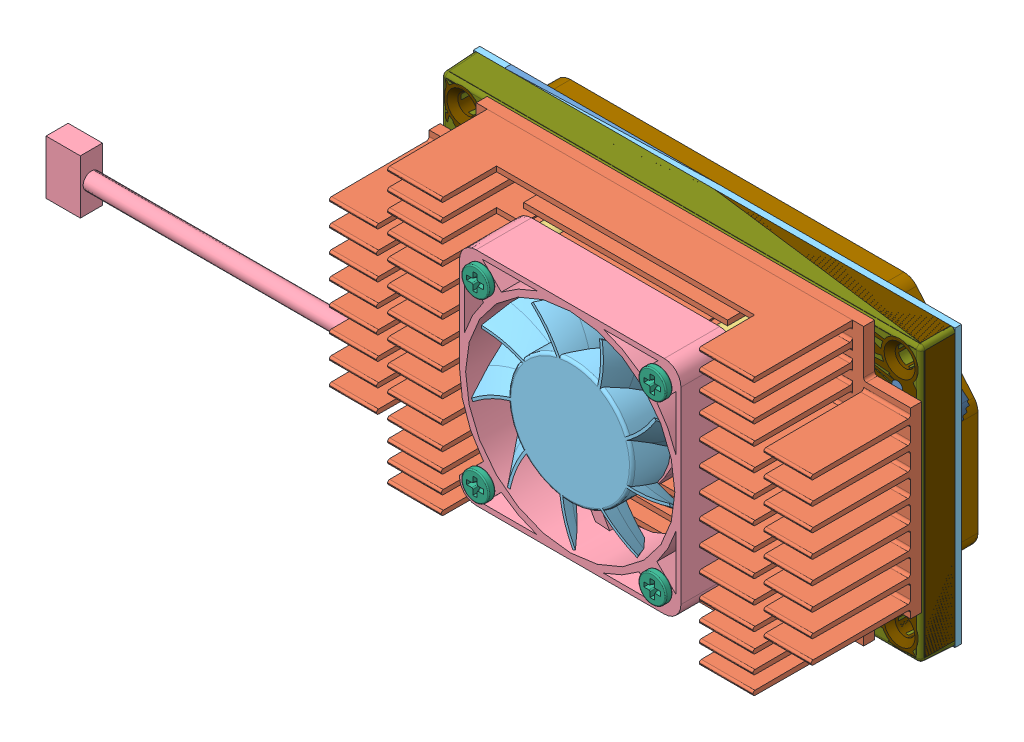
SolidWorks assembly JETSON-NEW_ASM, configuration Default. Lengths in mm. (continued)
Components (placement in the parent): (continued)
- 244-82180-1000-A03-10-12-15_ASM-1: 244-82180-1000-A03-10-12-15_ASM [Default] at origin size (87 50 8.3) (continued)
  - 039-0165-000_1-14: 039-0165-000_1 [Default] at (31.368 23.724 0) x (-1 0 0) z (0 0 -1) size (0.69 0.32 0.34)
  - 039-0165-000_1-15: 039-0165-000_1 [Default] at (30.473 23.719 0) x (-1 0 0) z (0 0 -1) size (0.69 0.32 0.34)
  - 195-2117-000_1-6: 195-2117-000_1 [Default] at (30.515 23.194 0) x (1 0 0) z (0 0 -1) size (0.69 0.32 0.31)
  - 039-0165-000_1-16: 039-0165-000_1 [Default] at (31.401 23.194 0) x (-1 0 0) z (0 0 -1) size (0.69 0.32 0.34)
  - 195-1636-000_1-21: 195-1636-000_1 [Default] at (67.75 12.2 0) x (0 -1 0) z (0 0 -1) size (0.69 0.32 0.31)
  - 039-0165-000_1-17: 039-0165-000_1 [Default] at (32.1 33 0) x (-1 0 0) z (0 0 -1) size (0.69 0.32 0.34)
  - 039-0165-000_1-18: 039-0165-000_1 [Default] at (33.713 34.804 0) x (0 1 0) z (0 0 -1) size (0.69 0.32 0.34)
  - 039-0165-000_1-19: 039-0165-000_1 [Default] at (32.583 23.814 0) x (-1 0 0) z (0 0 -1) size (0.69 0.32 0.34)
  - 039-0165-000_1-20: 039-0165-000_1 [Default] at (32.323 23.294 0) x (1 0 0) z (0 0 -1) size (0.69 0.32 0.34)
  - 195-1636-000_1-22: 195-1636-000_1 [Default] at (37.4 29.65 0) x (-1 0 0) z (0 0 -1) size (0.69 0.32 0.31)
  - 039-0165-000_1-21: 039-0165-000_1 [Default] at (11.65 14.4 0) x (1 0 0) z (0 0 -1) size (0.69 0.32 0.34)
  - 195-2006-000_1-6: 195-2006-000_1 [Default] at (11.65 13.85 0) x (1 0 0) z (0 0 -1) size (0.69 0.32 0.31)
  - 039-0165-000_1-22: 039-0165-000_1 [Default] at (32.5 41.35 0) x (0 -1 0) z (0 0 -1) size (0.69 0.32 0.34)
  - 039-0165-000_1-23: 039-0165-000_1 [Default] at (35.733 34.964 0) x (0 -1 0) z (0 0 -1) size (0.69 0.32 0.34)
  - 195-2005-000_1-8: 195-2005-000_1 [Default] at (32.265 27.36 0) x (-1 0 0) z (0 0 -1) size (0.69 0.32 0.31)
  - 195-1636-000_1-23: 195-1636-000_1 [Default] at (35.358 25.641 0) x (1 0 0) z (0 0 -1) size (0.69 0.32 0.31)
  - 039-0165-000_1-24: 039-0165-000_1 [Default] at (36.07 25.804 0) x (0 1 0) z (0 0 -1) size (0.69 0.32 0.34)
  - 039-0165-000_1-25: 039-0165-000_1 [Default] at (39.603 39.284 0) x (0 1 0) z (0 0 -1) size (0.69 0.32 0.34)
  - 039-0165-000_1-26: 039-0165-000_1 [Default] at (39.733 34.784 0) x (-1 0 0) z (0 0 -1) size (0.69 0.32 0.34)
  - 039-0165-000_1-27: 039-0165-000_1 [Default] at (40.473 23.854 0) x (0 1 0) z (0 0 -1) size (0.69 0.32 0.34)
  - 039-0165-000_1-28: 039-0165-000_1 [Default] at (37.453 39.204 0) x (-1 0 0) z (0 0 -1) size (0.69 0.32 0.34)
  - 195-1758-000_1-3: 195-1758-000_1 [Default] at (37.75 38.15 0) x (0 -1 0) z (0 0 -1) size (0.69 0.32 0.27)
  - 195-1758-000_1-4: 195-1758-000_1 [Default] at (37.8 35.75 0) x (0 -1 0) z (0 0 -1) size (0.69 0.32 0.27)
  - 039-0165-000_1-29: 039-0165-000_1 [Default] at (38.7 36 0) x (1 0 0) z (0 0 -1) size (0.69 0.32 0.34)
  - 039-0165-000_1-30: 039-0165-000_1 [Default] at (38.7 34.4 0) x (1 0 0) z (0 0 -1) size (0.69 0.32 0.34)
  - 039-0165-000_1-31: 039-0165-000_1 [Default] at (42 32.8 0) x (-1 0 0) z (0 0 -1) size (0.69 0.32 0.34)
  - 039-0165-000_1-32: 039-0165-000_1 [Default] at (39.75 33.05 0) x (0 1 0) z (0 0 -1) size (0.69 0.32 0.34)
  - 195-2005-000_1-9: 195-2005-000_1 [Default] at (40.728 29.454 0) x (0 -1 0) z (0 0 -1) size (0.69 0.32 0.31)
  - 195-1636-000_1-24: 195-1636-000_1 [Default] at (40.853 28.394 0) x (1 0 0) z (0 0 -1) size (0.69 0.32 0.31)
  - 039-0165-000_1-33: 039-0165-000_1 [Default] at (41.752 23.379 0) x (0 1 0) z (0 0 -1) size (0.69 0.32 0.34)
  - 195-2005-000_1-10: 195-2005-000_1 [Default] at (42.903 40.854 0) x (-1 0 0) z (0 0 -1) size (0.69 0.32 0.31)
  - 195-2006-000_1-7: 195-2006-000_1 [Default] at (42.753 39.054 0) x (0 -1 0) z (0 0 -1) size (0.69 0.32 0.31)
  - 195-2006-000_1-8: 195-2006-000_1 [Default] at (42.763 39.967 0) x (0 1 0) z (0 0 -1) size (0.69 0.32 0.31)
  - 039-0165-000_1-34: 039-0165-000_1 [Default] at (44.25 39.95 0) x (1 0 0) z (0 0 -1) size (0.69 0.32 0.34)
  - 039-0165-000_1-35: 039-0165-000_1 [Default] at (42.753 38.054 0) x (0 -1 0) z (0 0 -1) size (0.69 0.32 0.34)
  - 195-1636-000_1-25: 195-1636-000_1 [Default] at (42.9 35.2 0) x (0 -1 0) z (0 0 -1) size (0.69 0.32 0.31)
  - 039-0165-000_1-36: 039-0165-000_1 [Default] at (43.65 35.2 0) x (0 -1 0) z (0 0 -1) size (0.69 0.32 0.34)
  - 195-1636-000_1-26: 195-1636-000_1 [Default] at (41.4 34.05 0) x (1 0 0) z (0 0 -1) size (0.69 0.32 0.31)
  - 039-0165-000_1-37: 039-0165-000_1 [Default] at (43.7 34.15 0) x (0 -1 0) z (0 0 -1) size (0.69 0.32 0.34)
  - 039-0165-000_1-38: 039-0165-000_1 [Default] at (47.623 34.054 0) x (-1 0 0) z (0 0 -1) size (0.69 0.32 0.34)
  - 039-0165-000_1-39: 039-0165-000_1 [Default] at (48.447 33.88 0) x (0 -1 0) z (0 0 -1) size (0.69 0.32 0.34)
  - 195-2005-000_1-11: 195-2005-000_1 [Default] at (47.263 26.769 0) x (1 0 0) z (0 0 -1) size (0.69 0.32 0.31)
  - 039-0165-000_1-40: 039-0165-000_1 [Default] at (46.253 38.504 0) x (0 1 0) z (0 0 -1) size (0.69 0.32 0.34)
  - 039-0165-000_1-41: 039-0165-000_1 [Default] at (46.603 37.074 0) x (0 -1 0) z (0 0 -1) size (0.69 0.32 0.34)
  - 195-2002-000_1-1: 195-2002-000_1 [Default] at (46.55 34.9 0) x (1 0 0) z (0 0 -1) size (0.69 0.32 0.31)
  - 039-0165-000_1-42: 039-0165-000_1 [Default] at (47.15 32.9 0) x (1 0 0) z (0 0 -1) size (0.69 0.32 0.34)
  - 039-0165-000_1-43: 039-0165-000_1 [Default] at (44.25 38.9 0) x (1 0 0) z (0 0 -1) size (0.69 0.32 0.34)
  - 039-0165-000_1-44: 039-0165-000_1 [Default] at (43.853 36.604 0) x (-1 0 0) z (0 0 -1) size (0.69 0.32 0.34)
  - 039-0165-000_1-45: 039-0165-000_1 [Default] at (45.353 34.444 0) x (-1 0 0) z (0 0 -1) size (0.69 0.32 0.34)
  - 039-0165-000_1-46: 039-0165-000_1 [Default] at (45.5 32.55 0) x (0 -1 0) z (0 0 -1) size (0.69 0.32 0.34)
  - 039-0165-000_1-47: 039-0165-000_1 [Default] at (43.65 33.05 0) x (0 1 0) z (0 0 -1) size (0.69 0.32 0.34)
  - 195-1636-000_1-27: 195-1636-000_1 [Default] at (48.94 10.93 0) x (0 -1 0) z (0 0 -1) size (0.69 0.32 0.31)
  - 039-0165-000_1-48: 039-0165-000_1 [Default] at (50.928 40.754 0) x (1 0 0) z (0 0 -1) size (0.69 0.32 0.34)
  - 039-0165-000_1-49: 039-0165-000_1 [Default] at (49.163 33.855 0) x (0 -1 0) z (0 0 -1) size (0.69 0.32 0.34)
  - 039-0165-000_1-50: 039-0165-000_1 [Default] at (51.243 29.284 0) x (1 0 0) z (0 0 -1) size (0.69 0.32 0.34)
  - 039-0165-000_1-51: 039-0165-000_1 [Default] at (50.503 39.654 0) x (-1 0 0) z (0 0 -1) size (0.69 0.32 0.34)
  - 039-0165-000_1-52: 039-0165-000_1 [Default] at (50.503 38.954 0) x (-1 0 0) z (0 0 -1) size (0.69 0.32 0.34)
  - 039-0165-000_1-53: 039-0165-000_1 [Default] at (49.853 36.179 0) x (0 1 0) z (0 0 -1) size (0.69 0.32 0.34)
  - 039-0165-000_1-54: 039-0165-000_1 [Default] at (50.314 37.05 0) x (-1 0 0) z (0 0 -1) size (0.69 0.32 0.34)
  - 195-2002-000_1-2: 195-2002-000_1 [Default] at (47.45 34.9 0) x (-1 0 0) z (0 0 -1) size (0.69 0.32 0.31)
  - 039-0165-000_1-55: 039-0165-000_1 [Default] at (48.879 32.877 0) x (-1 0 0) z (0 0 -1) size (0.69 0.32 0.34)
  - 195-1636-000_1-28: 195-1636-000_1 [Default] at (48.34 10.93 0) x (0 -1 0) z (0 0 -1) size (0.69 0.32 0.31)
  - 035-0122-000_1-1: 035-0122-000_1 [Default] at (4.828 35.604 1.164) x (0 1 0) z (0 0 1) size (0.69 0.32 0.34)
  - 195-1636-000_1-29: 195-1636-000_1 [Default] at (4.753 32.979 1.164) x (-1 0 0) z (0 0 1) size (0.69 0.32 0.31)
  - 195-1636-000_1-30: 195-1636-000_1 [Default] at (4.512 32.738 1.164) x (0 1 0) z (0 0 1) size (0.69 0.32 0.31)
  - 035-0122-000_1-2: 035-0122-000_1 [Default] at (4.078 33.854 1.164) x (-1 0 0) z (0 0 1) size (0.69 0.32 0.34)
  - 195-1636-000_1-31: 195-1636-000_1 [Default] at (5.061 30.945 1.164) x (-1 0 0) z (0 0 1) size (0.69 0.32 0.31)
  - 130-0330-000_1-1: 130-0330-000_1 [Default] at (4.408 29.445 1.164) x (0 -1 0) z (0 0 1) size (0.69 0.32 0.34)
  - 035-0243-000_2-4: 035-0243-000_2 [Default] at (5.191 29.686 1.164) x (-1 0 0) z (0 0 1) size (0.69 0.32 0.34)
  - 195-2005-000_1-12: 195-2005-000_1 [Default] at (5.423 27.972 1.164) x (0 -1 0) z (0 0 1) size (0.69 0.32 0.31)
  - 195-2005-000_1-13: 195-2005-000_1 [Default] at (4.705 27.972 1.164) x (0 -1 0) z (0 0 1) size (0.69 0.32 0.31)
  - 039-0165-000_1-56: 039-0165-000_1 [Default] at (18.95 30.45 0) x (-1 0 0) z (0 0 -1) size (0.69 0.32 0.34)
  - 130-0330-000_1-2: 130-0330-000_1 [Default] at (3.596 35.184 1.164) x (-1 0 0) z (0 0 1) size (0.69 0.32 0.34)
  - 195-1636-000_1-32: 195-1636-000_1 [Default] at (4.533 25.324 1.164) x (0 1 0) z (0 0 1) size (0.69 0.32 0.31)
  - 035-0243-000_2-5: 035-0243-000_2 [Default] at (8.235 29.188 1.164) x (-1 0 0) z (0 0 1) size (0.69 0.32 0.34)
  - 195-2005-000_1-14: 195-2005-000_1 [Default] at (8.218 25.314 1.164) x (0 -1 0) z (0 0 1) size (0.69 0.32 0.31)
  - 195-1636-000_1-33: 195-1636-000_1 [Default] at (7.7 25.314 1.164) x (0 1 0) z (0 0 1) size (0.69 0.32 0.31)
  - 195-1636-000_1-34: 195-1636-000_1 [Default] at (8.736 25.314 1.164) x (0 1 0) z (0 0 1) size (0.69 0.32 0.31)
  - 195-1636-000_1-35: 195-1636-000_1 [Default] at (5.814 36.455 1.164) x (-1 0 0) z (0 0 1) size (0.69 0.32 0.31)
  - 035-0243-000_2-6: 035-0243-000_2 [Default] at (6.599 34.734 1.164) x (-1 0 0) z (0 0 1) size (0.69 0.32 0.34)
  - 035-0243-000_2-7: 035-0243-000_2 [Default] at (5.823 35.854 1.164) x (-1 0 0) z (0 0 1) size (0.69 0.32 0.34)
  - 195-1636-000_1-36: 195-1636-000_1 [Default] at (6.723 35.854 1.164) x (-1 0 0) z (0 0 1) size (0.69 0.32 0.31)
  - 035-0243-000_2-8: 035-0243-000_2 [Default] at (6.599 33.749 1.164) x (-1 0 0) z (0 0 1) size (0.69 0.32 0.34)
  - 035-0243-000_2-9: 035-0243-000_2 [Default] at (6.51 31.341 1.164) size (0.69 0.32 0.34)
  - 035-0243-000_2-10: 035-0243-000_2 [Default] at (6.787 32.049 1.164) x (0 -1 0) z (0 0 1) size (0.69 0.32 0.34)
  - 195-1636-000_1-37: 195-1636-000_1 [Default] at (6.269 32.049 1.164) x (0 -1 0) z (0 0 1) size (0.69 0.32 0.31)
  - 035-0122-000_1-3: 035-0122-000_1 [Default] at (5.803 30.204 1.164) x (-1 0 0) z (0 0 1) size (0.69 0.32 0.34)
  - 035-0122-000_1-4: 035-0122-000_1 [Default] at (5.703 29.004 1.164) x (-1 0 0) z (0 0 1) size (0.69 0.32 0.34)
  - 195-2005-000_1-15: 195-2005-000_1 [Default] at (6.108 27.972 1.164) x (0 -1 0) z (0 0 1) size (0.69 0.32 0.31)
  - 039-0165-000_1-57: 039-0165-000_1 [Default] at (9.35 17.8 0) x (0 -1 0) z (0 0 -1) size (0.69 0.32 0.34)
  - 195-1636-000_1-38: 195-1636-000_1 [Default] at (6.146 25.314 1.164) x (0 1 0) z (0 0 1) size (0.69 0.32 0.31)
  - 195-1636-000_1-39: 195-1636-000_1 [Default] at (6.664 25.314 1.164) x (0 1 0) z (0 0 1) size (0.69 0.32 0.31)
  - 195-1636-000_1-40: 195-1636-000_1 [Default] at (7.182 25.314 1.164) x (0 1 0) z (0 0 1) size (0.69 0.32 0.31)
  - 195-1636-000_1-41: 195-1636-000_1 [Default] at (5.628 25.314 1.164) x (0 1 0) z (0 0 1) size (0.69 0.32 0.31)
  - 195-2006-000_1-9: 195-2006-000_1 [Default] at (17.687 31.24 0) x (0 -1 0) z (0 0 -1) size (0.69 0.32 0.31)
  - 195-1636-000_1-42: 195-1636-000_1 [Default] at (5.103 37.229 1.164) x (0 -1 0) z (0 0 1) size (0.69 0.32 0.31)
  - 195-1636-000_1-43: 195-1636-000_1 [Default] at (5.103 36.747 1.164) x (0 1 0) z (0 0 1) size (0.69 0.32 0.31)
  - 035-0243-000_2-11: 035-0243-000_2 [Default] at (4.078 34.434 1.164) x (-1 0 0) z (0 0 1) size (0.69 0.32 0.34)
  - 130-0334-000_1-1: 130-0334-000_1 [Default] at (9.408 35.498 1.164) x (0 -1 0) z (0 0 1) size (0.69 0.32 0.34)
  - 035-0105-000_1-1: 035-0105-000_1 [Default] at (10.11 35.738 1.164) size (0.69 0.32 0.34)
  - 130-0280-000_1-1: 130-0280-000_1 [Default] at (9.959 34.495 1.164) x (0 -1 0) z (0 0 1) size (0.69 0.32 0.36)
  - 035-0105-000_1-2: 035-0105-000_1 [Default] at (8.706 35.739 1.164) size (0.69 0.32 0.34)
  - 130-0330-000_1-3: 130-0330-000_1 [Default] at (9.78 32.603 1.164) x (0 -1 0) z (0 0 1) size (0.69 0.32 0.34)
  - 035-0243-000_2-12: 035-0243-000_2 [Default] at (10.088 33.749 1.164) x (-1 0 0) z (0 0 1) size (0.69 0.32 0.34)
  - 130-0330-000_1-4: 130-0330-000_1 [Default] at (9.381 33.989 1.164) x (0 1 0) z (0 0 1) size (0.69 0.32 0.34)
  - 035-0105-000_1-3: 035-0105-000_1 [Default] at (9.009 32.844 1.164) size (0.69 0.32 0.34)
  - 035-0105-000_1-4: 035-0105-000_1 [Default] at (10.39 32.142 1.164) x (0 1 0) z (0 0 1) size (0.69 0.32 0.34)
  - 130-0334-000_1-2: 130-0334-000_1 [Default] at (9.861 31.66 1.164) x (0 -1 0) z (0 0 1) size (0.69 0.32 0.34)
  - 035-0105-000_1-5: 035-0105-000_1 [Default] at (9.343 31.66 1.164) x (0 1 0) z (0 0 1) size (0.69 0.32 0.34)
  - 130-0330-000_1-5: 130-0330-000_1 [Default] at (9.602 29.429 1.164) x (0 1 0) z (0 0 1) size (0.69 0.32 0.34)
  - 195-2005-000_1-16: 195-2005-000_1 [Default] at (10.223 27.779 1.164) size (0.69 0.32 0.31)
  - 195-1636-000_1-44: 195-1636-000_1 [Default] at (9.254 25.314 1.164) x (0 1 0) z (0 0 1) size (0.69 0.32 0.31)
  - 035-0122-000_1-5: 035-0122-000_1 [Default] at (7.483 37.064 1.164) x (0 -1 0) z (0 0 1) size (0.69 0.32 0.34)
  - 035-0243-000_2-13: 035-0243-000_2 [Default] at (7.483 35.613 1.164) x (0 -1 0) z (0 0 1) size (0.69 0.32 0.34)
  - 130-0298-000_1-2: 130-0298-000_1 [Default] at (8.358 34.495 1.164) x (0 -1 0) z (0 0 1) size (0.69 0.32 0.36)
  - 035-0122-000_1-6: 035-0122-000_1 [Default] at (8.004 35.549 1.164) x (0 -1 0) z (0 0 1) size (0.69 0.32 0.34)
  - 035-0122-000_1-7: 035-0122-000_1 [Default] at (8.043 32.844 1.164) size (0.69 0.32 0.34)
  - 035-0122-000_1-8: 035-0122-000_1 [Default] at (7.235 30.984 1.164) x (0 -1 0) z (0 0 1) size (0.69 0.32 0.34)
  - 035-0122-000_1-9: 035-0122-000_1 [Default] at (7.305 32.049 1.164) x (0 1 0) z (0 0 1) size (0.69 0.32 0.34)
  - 035-0243-000_2-14: 035-0243-000_2 [Default] at (8.235 30.222 1.164) x (-1 0 0) z (0 0 1) size (0.69 0.32 0.34)
  - 035-0122-000_1-10: 035-0122-000_1 [Default] at (10.495 37.647 1.164) size (0.69 0.32 0.34)
  - 035-0122-000_1-11: 035-0122-000_1 [Default] at (10.495 37.129 1.164) size (0.69 0.32 0.34)
  - 035-0105-000_1-6: 035-0105-000_1 [Default] at (10.562 32.844 1.164) size (0.69 0.32 0.34)
  - 039-0165-000_1-58: 039-0165-000_1 [Default] at (11.078 33.679 1.164) x (0 1 0) z (0 0 1) size (0.69 0.32 0.34)
  - 035-0243-000_2-15: 035-0243-000_2 [Default] at (10.523 29.188 1.164) x (-1 0 0) z (0 0 1) size (0.69 0.32 0.34)
  - 195-2337-000_1-1: 195-2337-000_1 [Default] at (14.912 30.106 1.164) x (0 1 0) z (0 0 1) size (0.69 0.32 0.31)
  - 035-0135-000_1-1: 035-0135-000_1 [Default] at (14.93 29.21 1.164) x (0 -1 0) z (0 0 1) size (0.69 0.32 0.34)
  - 195-2005-000_1-17: 195-2005-000_1 [Default] at (13.85 41.55 0) x (0 -1 0) z (0 0 -1) size (0.69 0.32 0.31)
  - 039-0165-000_1-59: 039-0165-000_1 [Default] at (13.85 40.55 0) x (0 -1 0) z (0 0 -1) size (0.69 0.32 0.34)
  - 035-0105-000_1-7: 035-0105-000_1 [Default] at (13.573 36.209 1.164) x (0 -1 0) z (0 0 1) size (0.69 0.32 0.34)
  - 035-0105-000_1-8: 035-0105-000_1 [Default] at (12.753 37.409 1.164) size (0.69 0.32 0.34)
  - 195-1636-000_1-45: 195-1636-000_1 [Default] at (13.621 34.372 0) x (0 1 0) z (0 0 -1) size (0.69 0.32 0.31)
  - 035-0135-000_1-2: 035-0135-000_1 [Default] at (13.038 28.694 1.164) x (-1 0 0) z (0 0 1) size (0.69 0.32 0.34)
  - 035-0234-000_2-1: 035-0234-000_2 [Default] at (14.085 37.68 1.164) x (-1 0 0) z (0 0 1) size (0.69 0.32 0.34)
  - 035-0122-000_1-12: 035-0122-000_1 [Default] at (14.106 36.209 1.164) x (0 1 0) z (0 0 1) size (0.69 0.32 0.34)
  - 130-0330-000_1-6: 130-0330-000_1 [Default] at (13.817 36.938 1.164) size (0.69 0.32 0.34)
  - 035-0122-000_1-13: 035-0122-000_1 [Default] at (15.525 36.204 1.164) x (0 1 0) z (0 0 1) size (0.69 0.32 0.34)
  - 039-0165-000_1-60: 039-0165-000_1 [Default] at (15.007 36.204 1.164) x (0 1 0) z (0 0 1) size (0.69 0.32 0.34)
  - 195-1636-000_1-46: 195-1636-000_1 [Default] at (17.087 17.723 0) x (1 0 0) z (0 0 -1) size (0.69 0.32 0.31)
  - 195-1636-000_1-47: 195-1636-000_1 [Default] at (17.1 16.02 0) x (1 0 0) z (0 0 -1) size (0.69 0.32 0.31)
  - 195-1636-000_1-48: 195-1636-000_1 [Default] at (17.05 16.57 0) x (1 0 0) z (0 0 -1) size (0.69 0.32 0.31)
  - 039-0165-000_1-61: 039-0165-000_1 [Default] at (15.397 32.956 0) x (0 -1 0) z (0 0 -1) size (0.69 0.32 0.34)
  - 039-0165-000_1-62: 039-0165-000_1 [Default] at (16.621 39.105 0) x (0 1 0) z (0 0 -1) size (0.69 0.32 0.34)
  - 195-2005-000_1-18: 195-2005-000_1 [Default] at (16.063 36.204 1.164) x (0 1 0) z (0 0 1) size (0.69 0.32 0.31)
  - 195-1636-000_1-49: 195-1636-000_1 [Default] at (17.087 18.25 0) x (1 0 0) z (0 0 -1) size (0.69 0.32 0.31)
  - 039-0199-000_1-1: 039-0199-000_1 [Default] at (16.451 29.906 1.164) x (0 -1 0) z (0 0 1) size (0.69 0.32 0.36)
  - 195-2117-000_1-7: 195-2117-000_1 [Default] at (19.3 11.7 0) x (0 1 0) z (0 0 -1) size (0.69 0.32 0.31)
  - 195-2117-000_1-8: 195-2117-000_1 [Default] at (18.55 17.19 0) x (1 0 0) z (0 0 -1) size (0.69 0.32 0.31)
  - 195-2005-000_1-19: 195-2005-000_1 [Default] at (18.588 36.204 1.164) x (0 1 0) z (0 0 1) size (0.69 0.32 0.31)
  - 195-1636-000_1-50: 195-1636-000_1 [Default] at (17.853 36.204 1.164) x (0 -1 0) z (0 0 1) size (0.69 0.32 0.31)
  - 195-1636-000_1-51: 195-1636-000_1 [Default] at (18.597 34.602 0) x (0 1 0) z (0 0 -1) size (0.69 0.32 0.31)
  - 195-1636-000_1-52: 195-1636-000_1 [Default] at (18.079 34.602 0) x (0 1 0) z (0 0 -1) size (0.69 0.32 0.31)
  - 195-1636-000_1-53: 195-1636-000_1 [Default] at (17.409 34.602 0) x (0 1 0) z (0 0 -1) size (0.69 0.32 0.31)
  - 195-2172-000_1-1: 195-2172-000_1 [Default] at (27.7 14.4 1.164) x (-1 0 0) z (0 0 1) size (0.69 0.32 0.31)
  - 195-2172-000_1-2: 195-2172-000_1 [Default] at (27.723 12.914 1.164) x (-1 0 0) z (0 0 1) size (0.69 0.32 0.31)
  - 195-2487-000_1-1: 195-2487-000_1 [Default] at (26.123 16.104 0) x (0 1 0) z (0 0 -1) size (0.69 0.32 0.31)
  - 195-2006-000_1-10: 195-2006-000_1 [Default] at (24.965 11.846 0) x (0 -1 0) z (0 0 -1) size (0.69 0.32 0.31)
  - 039-0165-000_1-63: 039-0165-000_1 [Default] at (12.35 19.25 0) x (-1 0 0) z (0 0 -1) size (0.69 0.32 0.34)
  - 039-0165-000_1-64: 039-0165-000_1 [Default] at (7.6 21.05 0) x (1 0 0) z (0 0 -1) size (0.69 0.32 0.34)
  - 035-0243-000_2-16: 035-0243-000_2 [Default] at (27.7 21.95 1.164) size (0.69 0.32 0.34)
  - 195-2506-000_1-3: 195-2506-000_1 [Default] at (27.7 16.9 1.164) x (-1 0 0) z (0 0 1) size (0.69 0.32 0.31)
  - 039-0165-000_1-65: 039-0165-000_1 [Default] at (31.213 15.274 0) x (1 0 0) z (0 0 -1) size (0.69 0.32 0.34)
  - 039-0165-000_1-66: 039-0165-000_1 [Default] at (31.903 14.494 0) x (0 1 0) z (0 0 -1) size (0.69 0.32 0.34)
  - 039-0165-000_1-67: 039-0165-000_1 [Default] at (31.183 14.754 0) x (-1 0 0) z (0 0 -1) size (0.69 0.32 0.34)
  - 039-0165-000_1-68: 039-0165-000_1 [Default] at (31.133 14.234 0) x (-1 0 0) z (0 0 -1) size (0.69 0.32 0.34)
  - 039-0165-000_1-69: 039-0165-000_1 [Default] at (31.713 13.704 0) x (-1 0 0) z (0 0 -1) size (0.69 0.32 0.34)
  - 035-0243-000_2-17: 035-0243-000_2 [Default] at (32.85 8.65 1.164) size (0.69 0.32 0.34)
  - 039-0165-000_1-70: 039-0165-000_1 [Default] at (30.533 21.774 0) x (1 0 0) z (0 0 -1) size (0.69 0.32 0.34)
  - 195-2004-000_1-1: 195-2004-000_1 [Default] at (30.109 20.345 0) x (1 0 0) z (0 0 -1) size (0.69 0.32 0.31)
  - 195-1636-000_1-54: 195-1636-000_1 [Default] at (30.003 19.574 0) x (0 1 0) z (0 0 -1) size (0.69 0.32 0.31)
  - 039-0165-000_1-71: 039-0165-000_1 [Default] at (34.778 14.474 0) x (0 1 0) z (0 0 -1) size (0.69 0.32 0.34)
  - 039-0165-000_1-72: 039-0165-000_1 [Default] at (35.296 14.474 0) x (0 1 0) z (0 0 -1) size (0.69 0.32 0.34)
  - 039-0165-000_1-73: 039-0165-000_1 [Default] at (32.323 22.184 0) x (1 0 0) z (0 0 -1) size (0.69 0.32 0.34)
  - 039-0165-000_1-74: 039-0165-000_1 [Default] at (32.323 21.124 0) x (1 0 0) z (0 0 -1) size (0.69 0.32 0.34)
  - 039-0165-000_1-75: 039-0165-000_1 [Default] at (32.323 21.644 0) x (1 0 0) z (0 0 -1) size (0.69 0.32 0.34)
  - 039-0165-000_1-76: 039-0165-000_1 [Default] at (32.323 20.034 0) x (1 0 0) z (0 0 -1) size (0.69 0.32 0.34)
  - 039-0165-000_1-77: 039-0165-000_1 [Default] at (32.323 20.564 0) x (1 0 0) z (0 0 -1) size (0.69 0.32 0.34)
  - 039-0165-000_1-78: 039-0165-000_1 [Default] at (32.323 19.514 0) x (1 0 0) z (0 0 -1) size (0.69 0.32 0.34)
  - 039-0165-000_1-79: 039-0165-000_1 [Default] at (32.323 17.394 0) x (1 0 0) z (0 0 -1) size (0.69 0.32 0.34)
  - 039-0165-000_1-80: 039-0165-000_1 [Default] at (32.323 16.794 0) x (1 0 0) z (0 0 -1) size (0.69 0.32 0.34)
  - 039-0165-000_1-81: 039-0165-000_1 [Default] at (32.323 16.274 0) x (1 0 0) z (0 0 -1) size (0.69 0.32 0.34)
  - 039-0165-000_1-82: 039-0165-000_1 [Default] at (32.323 15.744 0) x (1 0 0) z (0 0 -1) size (0.69 0.32 0.34)
  - 039-0165-000_1-83: 039-0165-000_1 [Default] at (32.323 15.214 0) x (1 0 0) z (0 0 -1) size (0.69 0.32 0.34)
  - 039-0165-000_1-84: 039-0165-000_1 [Default] at (32.954 14.494 0) x (0 1 0) z (0 0 -1) size (0.69 0.32 0.34)
  - 039-0165-000_1-85: 039-0165-000_1 [Default] at (32.436 14.494 0) x (0 1 0) z (0 0 -1) size (0.69 0.32 0.34)
  - 195-2172-000_1-3: 195-2172-000_1 [Default] at (34.65 10.1 1.164) x (0 -1 0) z (0 0 1) size (0.69 0.32 0.31)
  - 035-0243-000_2-18: 035-0243-000_2 [Default] at (33.323 10.09 1.164) x (0 1 0) z (0 0 1) size (0.69 0.32 0.34)
  - 039-0165-000_1-86: 039-0165-000_1 [Default] at (31.433 21.764 0) x (-1 0 0) z (0 0 -1) size (0.69 0.32 0.34)
  - 039-0165-000_1-87: 039-0165-000_1 [Default] at (32.323 22.724 0) x (1 0 0) z (0 0 -1) size (0.69 0.32 0.34)
  - 039-0165-000_1-88: 039-0165-000_1 [Default] at (31.363 20.344 0) x (-1 0 0) z (0 0 -1) size (0.69 0.32 0.34)
  - 039-0165-000_1-89: 039-0165-000_1 [Default] at (38.068 14.474 0) x (0 1 0) z (0 0 -1) size (0.69 0.32 0.34)
  - 039-0165-000_1-90: 039-0165-000_1 [Default] at (37.55 14.474 0) x (0 1 0) z (0 0 -1) size (0.69 0.32 0.34)
  - 039-0165-000_1-91: 039-0165-000_1 [Default] at (38.586 14.474 0) x (0 1 0) z (0 0 -1) size (0.69 0.32 0.34)
  - 039-0165-000_1-92: 039-0165-000_1 [Default] at (39.104 14.474 0) x (0 1 0) z (0 0 -1) size (0.69 0.32 0.34)
  - 195-2631-000_1-1: 195-2631-000_1 [Default] at (38.639 10.011 1.164) x (0 -1 0) z (0 0 1) size (0.69 0.32 0.31)
  - 195-1636-000_1-55: 195-1636-000_1 [Default] at (38.36 9.734 1.164) x (-1 0 0) z (0 0 1) size (0.69 0.32 0.31)
  - 195-1636-000_1-56: 195-1636-000_1 [Default] at (38.36 10.292 1.164) x (-1 0 0) z (0 0 1) size (0.69 0.32 0.31)
  - 039-0165-000_1-93: 039-0165-000_1 [Default] at (35.814 14.474 0) x (0 1 0) z (0 0 -1) size (0.69 0.32 0.34)
  - 039-0165-000_1-94: 039-0165-000_1 [Default] at (34.172 14.474 0) x (0 1 0) z (0 0 -1) size (0.69 0.32 0.34)
  - 039-0165-000_1-95: 039-0165-000_1 [Default] at (40.833 17.074 0) x (-1 0 0) z (0 0 -1) size (0.69 0.32 0.34)
  - 039-0165-000_1-96: 039-0165-000_1 [Default] at (40.833 16.034 0) x (-1 0 0) z (0 0 -1) size (0.69 0.32 0.34)
  - 039-0165-000_1-97: 039-0165-000_1 [Default] at (40.833 15.514 0) x (-1 0 0) z (0 0 -1) size (0.69 0.32 0.34)
  - 039-0165-000_1-98: 039-0165-000_1 [Default] at (40.843 14.994 0) x (-1 0 0) z (0 0 -1) size (0.69 0.32 0.34)
  - 039-0165-000_1-99: 039-0165-000_1 [Default] at (40.843 14.474 0) x (-1 0 0) z (0 0 -1) size (0.69 0.32 0.34)
  - 039-0165-000_1-100: 039-0165-000_1 [Default] at (42.073 13.724 0) x (0 1 0) z (0 0 -1) size (0.69 0.32 0.34)
  - 039-0165-000_1-101: 039-0165-000_1 [Default] at (41.553 13.724 0) x (0 -1 0) z (0 0 -1) size (0.69 0.32 0.34)
  - 039-0165-000_1-102: 039-0165-000_1 [Default] at (41.033 13.724 0) x (0 -1 0) z (0 0 -1) size (0.69 0.32 0.34)
  - 195-2363-000_1-1: 195-2363-000_1 [Default] at (40.25 10.1 1.164) x (0 -1 0) z (0 0 1) size (0.69 0.32 0.31)
  - 195-2631-000_1-2: 195-2631-000_1 [Default] at (41.863 10.104 1.164) x (0 1 0) z (0 0 1) size (0.69 0.32 0.31)
  - 195-1636-000_1-57: 195-1636-000_1 [Default] at (10.8 12.1 0) x (0 -1 0) z (0 0 -1) size (0.69 0.32 0.31)
  - 039-0165-000_1-103: 039-0165-000_1 [Default] at (40.14 14.474 0) x (0 1 0) z (0 0 -1) size (0.69 0.32 0.34)
  - 039-0165-000_1-104: 039-0165-000_1 [Default] at (39.622 14.474 0) x (0 1 0) z (0 0 -1) size (0.69 0.32 0.34)
  - 195-2631-000_1-3: 195-2631-000_1 [Default] at (39.729 10.094 1.164) x (0 -1 0) z (0 0 1) size (0.69 0.32 0.31)
  - 039-0165-000_1-105: 039-0165-000_1 [Default] at (64.72 13.486 0) x (0 -1 0) z (0 0 -1) size (0.69 0.32 0.34)
  - 195-1636-000_1-58: 195-1636-000_1 [Default] at (43.938 22.284 0) x (0 1 0) z (0 0 -1) size (0.69 0.32 0.31)
  - 195-2363-000_1-2: 195-2363-000_1 [Default] at (42.35 11.2 0) x (0 -1 0) z (0 0 -1) size (0.69 0.32 0.31)
  - 195-2118-000_1-4: 195-2118-000_1 [Default] at (43.33 10.106 1.164) x (0 1 0) z (0 0 1) size (0.69 0.32 0.31)
  - 195-2118-000_1-5: 195-2118-000_1 [Default] at (43.89 10.106 1.164) x (0 1 0) z (0 0 1) size (0.69 0.32 0.31)
  - 035-0243-000_2-19: 035-0243-000_2 [Default] at (48.1 10.2 1.164) size (0.69 0.32 0.34)
  - 195-2006-000_1-11: 195-2006-000_1 [Default] at (57.9 10.05 1.164) size (0.69 0.32 0.31)
  - 039-0165-000_1-106: 039-0165-000_1 [Default] at (40.833 22.304 0) x (-1 0 0) z (0 0 -1) size (0.69 0.32 0.34)
  - 039-0165-000_1-107: 039-0165-000_1 [Default] at (41.493 20.984 0) x (0 -1 0) z (0 0 -1) size (0.69 0.32 0.34)
  - 039-0165-000_1-108: 039-0165-000_1 [Default] at (40.833 21.774 0) x (-1 0 0) z (0 0 -1) size (0.69 0.32 0.34)
  - 195-2171-000_1-1: 195-2171-000_1 [Default] at (42.013 20.824 0) x (0 -1 0) z (0 0 -1) size (0.69 0.32 0.31)
  - 195-2171-000_1-2: 195-2171-000_1 [Default] at (41.75 19.276 0) x (-1 0 0) z (0 0 -1) size (0.69 0.32 0.31)
  - 195-2006-000_1-12: 195-2006-000_1 [Default] at (67.73 15.666 0) x (0 1 0) z (0 0 -1) size (0.69 0.32 0.31)
  - 039-0165-000_1-109: 039-0165-000_1 [Default] at (64.03 15.576 0) x (0 -1 0) z (0 0 -1) size (0.69 0.32 0.34)
  - 195-1636-000_1-59: 195-1636-000_1 [Default] at (45.55 15.15 1.164) x (0 -1 0) z (0 0 1) size (0.69 0.32 0.31)
  - 035-0243-000_2-20: 035-0243-000_2 [Default] at (44.45 20.9 0) x (1 0 0) z (0 0 -1) size (0.69 0.32 0.34)
  - 039-0165-000_1-110: 039-0165-000_1 [Default] at (58.53 35.436 0) x (0 1 0) z (0 0 -1) size (0.69 0.32 0.34)
  - 195-1636-000_1-60: 195-1636-000_1 [Default] at (58.79 33.596 0) x (0 1 0) z (0 0 -1) size (0.69 0.32 0.31)
  - 195-1636-000_1-61: 195-1636-000_1 [Default] at (56.903 40.239 0) x (-1 0 0) z (0 0 -1) size (0.69 0.32 0.31)
  - 039-0165-000_1-111: 039-0165-000_1 [Default] at (57.503 37.784 0) x (0 1 0) z (0 0 -1) size (0.69 0.32 0.34)
  - 195-2469-000_1-1: 195-2469-000_1 [Default] at (57.403 38.754 0) x (0 -1 0) z (0 0 -1) size (0.69 0.32 0.31)
  - 195-1636-000_1-62: 195-1636-000_1 [Default] at (57.19 37.076 0) x (-1 0 0) z (0 0 -1) size (0.69 0.32 0.31)
  - 195-1636-000_1-63: 195-1636-000_1 [Default] at (56.433 18.954 0) x (0 -1 0) z (0 0 -1) size (0.69 0.32 0.31)
  - 195-1636-000_1-64: 195-1636-000_1 [Default] at (56.153 17.514 0) x (1 0 0) z (0 0 -1) size (0.69 0.32 0.31)
  - 195-2006-000_1-13: 195-2006-000_1 [Default] at (56.153 18.064 0) x (1 0 0) z (0 0 -1) size (0.69 0.32 0.31)
  - 195-1636-000_1-65: 195-1636-000_1 [Default] at (56.153 16.294 0) x (-1 0 0) z (0 0 -1) size (0.69 0.32 0.31)
  - 195-2005-000_1-20: 195-2005-000_1 [Default] at (55.41 37.136 0) x (-1 0 0) z (0 0 -1) size (0.69 0.32 0.31)
  - 195-2005-000_1-21: 195-2005-000_1 [Default] at (54.515 37.047 0) x (1 0 0) z (0 0 -1) size (0.69 0.32 0.31)
  - 195-2004-000_1-2: 195-2004-000_1 [Default] at (54.515 36.527 0) x (1 0 0) z (0 0 -1) size (0.69 0.32 0.31)
  - 195-2004-000_1-3: 195-2004-000_1 [Default] at (54.515 36.007 0) x (1 0 0) z (0 0 -1) size (0.69 0.32 0.31)
  - 195-1636-000_1-66: 195-1636-000_1 [Default] at (56.3 37.076 0) x (1 0 0) z (0 0 -1) size (0.69 0.32 0.31)
  - 195-1636-000_1-67: 195-1636-000_1 [Default] at (69.95 41.15 0) x (-1 0 0) z (0 0 -1) size (0.69 0.32 0.31)
  - 039-0165-000_1-112: 039-0165-000_1 [Default] at (55.853 18.829 0) x (0 1 0) z (0 0 -1) size (0.69 0.32 0.34)
  - 195-2005-000_1-22: 195-2005-000_1 [Default] at (55.328 18.829 0) x (0 -1 0) z (0 0 -1) size (0.69 0.32 0.31)
  - 195-2173-000_1-1: 195-2173-000_1 [Default] at (55.063 17.794 0) x (-1 0 0) z (0 0 -1) size (0.69 0.32 0.31)
  - 195-2173-000_1-2: 195-2173-000_1 [Default] at (55.083 17.234 0) x (1 0 0) z (0 0 -1) size (0.69 0.32 0.31)
  - 039-0165-000_1-113: 039-0165-000_1 [Default] at (60.953 36.318 0) x (0 -1 0) z (0 0 -1) size (0.69 0.32 0.34)
  - 039-0165-000_1-114: 039-0165-000_1 [Default] at (59.253 34.954 0) x (1 0 0) z (0 0 -1) size (0.69 0.32 0.34)
  - 195-1636-000_1-68: 195-1636-000_1 [Default] at (59.32 33.596 0) x (0 1 0) z (0 0 -1) size (0.69 0.32 0.31)
  - 195-1636-000_1-69: 195-1636-000_1 [Default] at (59.85 33.596 0) x (0 1 0) z (0 0 -1) size (0.69 0.32 0.31)
  - 195-1636-000_1-70: 195-1636-000_1 [Default] at (61.26 31.736 0) x (-1 0 0) z (0 0 -1) size (0.69 0.32 0.31)
  - 195-1636-000_1-71: 195-1636-000_1 [Default] at (61.26 31.206 0) x (-1 0 0) z (0 0 -1) size (0.69 0.32 0.31)
  - 195-2005-000_1-23: 195-2005-000_1 [Default] at (58.65 38.25 0) x (0 1 0) z (0 0 -1) size (0.69 0.32 0.31)
  - 195-1636-000_1-72: 195-1636-000_1 [Default] at (58.103 37.754 0) x (0 -1 0) z (0 0 -1) size (0.69 0.32 0.31)
  - 039-0165-000_1-115: 039-0165-000_1 [Default] at (57.953 38.754 0) x (0 -1 0) z (0 0 -1) size (0.69 0.32 0.34)
  - 039-0165-000_1-116: 039-0165-000_1 [Default] at (58.08 36.986 0) x (1 0 0) z (0 0 -1) size (0.69 0.32 0.34)
  - 039-0165-000_1-117: 039-0165-000_1 [Default] at (58.06 36.446 0) x (1 0 0) z (0 0 -1) size (0.69 0.32 0.34)
  - 195-2005-000_1-24: 195-2005-000_1 [Default] at (64.55 39 0) x (0 -1 0) z (0 0 -1) size (0.69 0.32 0.31)
  - 195-1636-000_1-73: 195-1636-000_1 [Default] at (63.9 37.95 0) x (0 1 0) z (0 0 -1) size (0.69 0.32 0.31)
  - 195-2117-000_1-9: 195-2117-000_1 [Default] at (61.95 37.6 0) x (0 1 0) z (0 0 -1) size (0.69 0.32 0.31)
  - 195-2350-000_1-1: 195-2350-000_1 [Default] at (62.2 35.7 0) x (1 0 0) z (0 0 -1) size (0.69 0.32 0.31)
  - 195-1636-000_1-74: 195-1636-000_1 [Default] at (61.31 33.856 0) x (1 0 0) z (0 0 -1) size (0.69 0.32 0.31)
  - 195-1636-000_1-75: 195-1636-000_1 [Default] at (61.31 33.326 0) x (1 0 0) z (0 0 -1) size (0.69 0.32 0.31)
  - 035-0122-000_1-14: 035-0122-000_1 [Default] at (61.585 32.427 1.164) x (-1 0 0) z (0 0 1) size (0.69 0.32 0.34)
  - 195-1636-000_1-76: 195-1636-000_1 [Default] at (61.31 32.796 0) x (1 0 0) z (0 0 -1) size (0.69 0.32 0.31)
  - 195-2171-000_1-3: 195-2171-000_1 [Default] at (61.98 31.446 0) x (0 1 0) z (0 0 -1) size (0.69 0.32 0.31)
  - 195-2171-000_1-4: 195-2171-000_1 [Default] at (62.7 31.736 0) x (-1 0 0) z (0 0 -1) size (0.69 0.32 0.31)
  - 195-2171-000_1-5: 195-2171-000_1 [Default] at (62.7 31.206 0) x (-1 0 0) z (0 0 -1) size (0.69 0.32 0.31)
  - 195-2006-000_1-14: 195-2006-000_1 [Default] at (61.35 17 0) x (-1 0 0) z (0 0 -1) size (0.69 0.32 0.31)
  - 195-2006-000_1-15: 195-2006-000_1 [Default] at (67.003 18.404 0) x (1 0 0) z (0 0 -1) size (0.69 0.32 0.31)
  - 195-1636-000_1-77: 195-1636-000_1 [Default] at (63.1 35.25 0) x (1 0 0) z (0 0 -1) size (0.69 0.32 0.31)
  - 195-2006-000_1-16: 195-2006-000_1 [Default] at (60.735 35.528 0) x (1 0 0) z (0 0 -1) size (0.69 0.32 0.31)
  - 195-2005-000_1-25: 195-2005-000_1 [Default] at (70.6 26.95 0) x (0 1 0) z (0 0 -1) size (0.69 0.32 0.31)
  - 195-1636-000_1-78: 195-1636-000_1 [Default] at (69 26.8 0) x (1 0 0) z (0 0 -1) size (0.69 0.32 0.31)
  - 195-2005-000_1-26: 195-2005-000_1 [Default] at (68.818 25.999 0) x (0 -1 0) z (0 0 -1) size (0.69 0.32 0.31)
  - 195-2173-000_1-3: 195-2173-000_1 [Default] at (68.073 25.764 0) x (-1 0 0) z (0 0 -1) size (0.69 0.32 0.31)
  - 195-1636-000_1-79: 195-1636-000_1 [Default] at (68.053 24.804 0) x (0 1 0) z (0 0 -1) size (0.69 0.32 0.31)
  - 195-2006-000_1-17: 195-2006-000_1 [Default] at (69.153 24.484 0) x (0 -1 0) z (0 0 -1) size (0.69 0.32 0.31)
  - 195-1636-000_1-80: 195-1636-000_1 [Default] at (68.913 25.224 0) x (1 0 0) z (0 0 -1) size (0.69 0.32 0.31)
  - 195-1636-000_1-81: 195-1636-000_1 [Default] at (68.603 24.484 0) x (0 -1 0) z (0 0 -1) size (0.69 0.32 0.31)
  - 035-0135-000_1-3: 035-0135-000_1 [Default] at (69.153 19.404 0) x (0 -1 0) z (0 0 -1) size (0.69 0.32 0.34)
  - 195-2274-000_1-1: 195-2274-000_1 [Default] at (68.553 19.404 0) x (0 -1 0) z (0 0 -1) size (0.69 0.32 0.31)
  - 039-0219-000_1-1: 039-0219-000_1 [Default] at (67.753 18.304 0) x (0 -1 0) z (0 0 -1) size (0.69 0.32 0.34)
  - 035-0135-000_1-4: 035-0135-000_1 [Default] at (68.653 18.604 0) x (1 0 0) z (0 0 -1) size (0.69 0.32 0.34)
  - 195-2173-000_1-4: 195-2173-000_1 [Default] at (67.133 25.764 0) x (1 0 0) z (0 0 -1) size (0.69 0.32 0.31)
  - 195-2004-000_1-4: 195-2004-000_1 [Default] at (18.25 37.45 0) x (0 1 0) z (0 0 -1) size (0.69 0.32 0.31)
  - 195-2004-000_1-5: 195-2004-000_1 [Default] at (18.8 37.45 0) x (0 1 0) z (0 0 -1) size (0.69 0.32 0.31)
  - 195-1636-000_1-82: 195-1636-000_1 [Default] at (41.75 9 1.164) x (0 -1 0) z (0 0 1) size (0.69 0.32 0.31)
  - 195-2459-000_1-1: 195-2459-000_1 [Default] at (70.675 24.972 0) x (0 1 0) z (0 0 -1) size (0.69 0.32 0.31)
  - 195-1636-000_1-83: 195-1636-000_1 [Default] at (70.053 24.254 0) x (1 0 0) z (0 0 -1) size (0.69 0.32 0.31)
  - 039-0165-000_1-118: 039-0165-000_1 [Default] at (69.903 24.854 0) x (1 0 0) z (0 0 -1) size (0.69 0.32 0.34)
  - 195-1636-000_1-84: 195-1636-000_1 [Default] at (70.753 20.604 0) x (0 -1 0) z (0 0 -1) size (0.69 0.32 0.31)
  - 035-0135-000_1-5: 035-0135-000_1 [Default] at (70.553 19.284 0) x (1 0 0) z (0 0 -1) size (0.69 0.32 0.34)
  - 195-2172-000_1-4: 195-2172-000_1 [Default] at (70.553 19.804 0) x (1 0 0) z (0 0 -1) size (0.69 0.32 0.31)
  - 035-0135-000_1-6: 035-0135-000_1 [Default] at (69.753 19.404 0) x (0 -1 0) z (0 0 -1) size (0.69 0.32 0.34)
  - 195-2172-000_1-5: 195-2172-000_1 [Default] at (70.253 18.004 0) x (1 0 0) z (0 0 -1) size (0.69 0.32 0.31)
  - 195-1636-000_1-85: 195-1636-000_1 [Default] at (70.253 18.604 0) x (1 0 0) z (0 0 -1) size (0.69 0.32 0.31)
  - 035-0135-000_1-7: 035-0135-000_1 [Default] at (71.25 18 0) x (1 0 0) z (0 0 -1) size (0.69 0.32 0.34)
  - 215-0247-000_1-4: 215-0247-000_1 [Default] at (68.9 33 0) x (0 1 0) z (0 0 -1) size (0.69 0.32 0.33)
  - 215-0247-000_1-5: 215-0247-000_1 [Default] at (73.4 30.6 0) x (1 0 0) z (0 0 -1) size (0.69 0.32 0.33)
  - 195-2319-000_1-1: 195-2319-000_1 [Default] at (70.953 23.922 0) x (-1 0 0) z (0 0 -1) size (0.69 0.32 0.31)
  - 039-0199-000_1-2: 039-0199-000_1 [Default] at (70.953 22.804 0) x (1 0 0) z (0 0 -1) size (0.69 0.32 0.36)
  - 195-2299-000_1-1: 195-2299-000_1 [Default] at (71.853 22.804 0) x (-1 0 0) z (0 0 -1) size (0.69 0.32 0.31)
  - 195-2289-000_1-1: 195-2289-000_1 [Default] at (70.953 23.404 0) x (1 0 0) z (0 0 -1) size (0.69 0.32 0.31)
  - 195-1636-000_1-86: 195-1636-000_1 [Default] at (71.853 23.404 0) x (1 0 0) z (0 0 -1) size (0.69 0.32 0.31)
  - 032-0335-000_1-1: 032-0335-000_1 [Default] at (71.553 20.804 0) x (-1 0 0) z (0 0 -1) size (0.69 0.32 0.34)
  - 195-2173-000_1-5: 195-2173-000_1 [Default] at (70.953 21.404 0) x (-1 0 0) z (0 0 -1) size (0.69 0.32 0.31)
  - 195-2061-000_1-1: 195-2061-000_1 [Default] at (71.853 21.404 0) x (-1 0 0) z (0 0 -1) size (0.69 0.32 0.31)
  - 195-2548-000_1-1: 195-2548-000_1 [Default] at (70.953 22.204 0) x (1 0 0) z (0 0 -1) size (0.69 0.32 0.31)
  - 039-0165-000_1-119: 039-0165-000_1 [Default] at (71.853 22.204 0) x (1 0 0) z (0 0 -1) size (0.69 0.32 0.34)
  - 195-1636-000_1-87: 195-1636-000_1 [Default] at (72.5 19.9 0) x (1 0 0) z (0 0 -1) size (0.69 0.32 0.31)
  - 195-2003-000_1-1: 195-2003-000_1 [Default] at (71.25 18.6 0) x (1 0 0) z (0 0 -1) size (0.69 0.32 0.31)
  - 036-0107-000_1-1: 036-0107-000_1 [Default] at (71.553 19.304 0) x (1 0 0) z (0 0 -1) size (0.69 0.32 0.31)
  - 195-1636-000_1-88: 195-1636-000_1 [Default] at (71.553 19.904 0) x (1 0 0) z (0 0 -1) size (0.69 0.32 0.31)
  - 195-1636-000_1-89: 195-1636-000_1 [Default] at (72.5 19.3 0) x (1 0 0) z (0 0 -1) size (0.69 0.32 0.31)
  - 195-2003-000_1-2: 195-2003-000_1 [Default] at (72.5 20.45 0) x (1 0 0) z (0 0 -1) size (0.69 0.32 0.31)
  - 215-0247-000_1-6: 215-0247-000_1 [Default] at (74.5 30.3 0) x (1 0 0) z (0 0 -1) size (0.69 0.32 0.33)
  - 215-0247-000_1-7: 215-0247-000_1 [Default] at (77.75 33.4 0) x (1 0 0) z (0 0 -1) size (0.69 0.32 0.33)
  - 195-1636-000_1-90: 195-1636-000_1 [Default] at (74.65 29.5 0) x (0 1 0) z (0 0 -1) size (0.69 0.32 0.31)
  - 215-0247-000_1-8: 215-0247-000_1 [Default] at (73.55 31.15 0) x (-1 0 0) z (0 0 -1) size (0.69 0.32 0.33)
  - 195-1636-000_1-91: 195-1636-000_1 [Default] at (74.55 37.6 0) x (0 -1 0) z (0 0 -1) size (0.69 0.32 0.31)
  - 035-0243-000_2-21: 035-0243-000_2 [Default] at (21.1 29.15 1.164) x (0 -1 0) z (0 0 1) size (0.69 0.32 0.34)
  - 035-0243-000_2-22: 035-0243-000_2 [Default] at (22.3 24.7 1.164) x (-1 0 0) z (0 0 1) size (0.69 0.32 0.34)
  - 195-2004-000_1-6: 195-2004-000_1 [Default] at (18.35 20.85 1.164) size (0.69 0.32 0.31)
  - 195-2004-000_1-7: 195-2004-000_1 [Default] at (18.35 21.4 1.164) size (0.69 0.32 0.31)
  - 195-2057-000_1-1: 195-2057-000_1 [Default] at (26.4 22.45 1.164) x (0 -1 0) z (0 0 1) size (0.69 0.32 0.31)
  - 195-2117-000_1-10: 195-2117-000_1 [Default] at (17.2 23.15 0) x (1 0 0) z (0 0 -1) size (0.69 0.32 0.31)
  - 195-2117-000_1-11: 195-2117-000_1 [Default] at (17.2 24.25 0) x (1 0 0) z (0 0 -1) size (0.69 0.32 0.31)
  - 195-2117-000_1-12: 195-2117-000_1 [Default] at (18.55 15.5 0) x (1 0 0) z (0 0 -1) size (0.69 0.32 0.31)
  - 195-2117-000_1-13: 195-2117-000_1 [Default] at (17.6 15.5 0) x (1 0 0) z (0 0 -1) size (0.69 0.32 0.31)
  - 195-2117-000_1-14: 195-2117-000_1 [Default] at (17.6 17.19 0) x (1 0 0) z (0 0 -1) size (0.69 0.32 0.31)
  - 195-1636-000_1-92: 195-1636-000_1 [Default] at (19.785 34.602 0) x (0 1 0) z (0 0 -1) size (0.69 0.32 0.31)
  - 195-1636-000_1-93: 195-1636-000_1 [Default] at (19.267 34.602 0) x (0 1 0) z (0 0 -1) size (0.69 0.32 0.31)
  - 195-1636-000_1-94: 195-1636-000_1 [Default] at (51.7 24.8 0) x (0 1 0) z (0 0 -1) size (0.69 0.32 0.31)
  - 035-0243-000_2-23: 035-0243-000_2 [Default] at (48.05 23.5 1.164) x (0 1 0) z (0 0 1) size (0.69 0.32 0.34)
  - 039-0165-000_1-120: 039-0165-000_1 [Default] at (41.543 22.374 0) x (0 -1 0) z (0 0 -1) size (0.69 0.32 0.34)
  - 039-0165-000_1-121: 039-0165-000_1 [Default] at (40.833 22.824 0) x (-1 0 0) z (0 0 -1) size (0.69 0.32 0.34)
  - 195-2007-000_1-1: 195-2007-000_1 [Default] at (18.65 12.6 0) x (0 -1 0) z (0 0 -1) size (0.69 0.32 0.31)
  - 195-1636-000_1-95: 195-1636-000_1 [Default] at (-0.85 36.75 1.164) x (-1 0 0) z (0 0 1) size (0.69 0.32 0.31)
  - 035-0243-000_2-24: 035-0243-000_2 [Default] at (-0.1 36.5 1.164) x (0 -1 0) z (0 0 1) size (0.69 0.32 0.34)
  - 035-0105-000_1-9: 035-0105-000_1 [Default] at (0.65 36.75 1.164) size (0.69 0.32 0.34)
  - 195-1636-000_1-96: 195-1636-000_1 [Default] at (-0.85 31.15 1.164) x (-1 0 0) z (0 0 1) size (0.69 0.32 0.31)
  - 035-0243-000_2-25: 035-0243-000_2 [Default] at (-0.1 30.9 1.164) x (0 -1 0) z (0 0 1) size (0.69 0.32 0.34)
  - 035-0105-000_1-10: 035-0105-000_1 [Default] at (0.65 31.15 1.164) size (0.69 0.32 0.34)
  - 035-0122-000_1-15: 035-0122-000_1 [Default] at (57.665 22.463 0) x (0 -1 0) z (0 0 -1) size (0.69 0.32 0.34)
  - 195-2566-000_1-1: 195-2566-000_1 [Default] at (31.05 10.1 1.164) x (0 -1 0) z (0 0 1) size (0.69 0.32 0.31)
  - 195-1636-000_1-97: 195-1636-000_1 [Default] at (64.54 30.986 0) x (-1 0 0) z (0 0 -1) size (0.69 0.32 0.31)
  - 195-1636-000_1-98: 195-1636-000_1 [Default] at (63.6 30.986 0) x (1 0 0) z (0 0 -1) size (0.69 0.32 0.31)
  - 195-1636-000_1-99: 195-1636-000_1 [Default] at (62.7 32.266 0) x (-1 0 0) z (0 0 -1) size (0.69 0.32 0.31)
  - 195-1636-000_1-100: 195-1636-000_1 [Default] at (61.26 32.266 0) x (-1 0 0) z (0 0 -1) size (0.69 0.32 0.31)
  - 036-0107-000_1-2: 036-0107-000_1 [Default] at (64.28 32.246 0) x (1 0 0) z (0 0 -1) size (0.69 0.32 0.31)
  - 195-2566-000_1-2: 195-2566-000_1 [Default] at (45.8 23.3 1.164) x (0 1 0) z (0 0 1) size (0.69 0.32 0.31)
